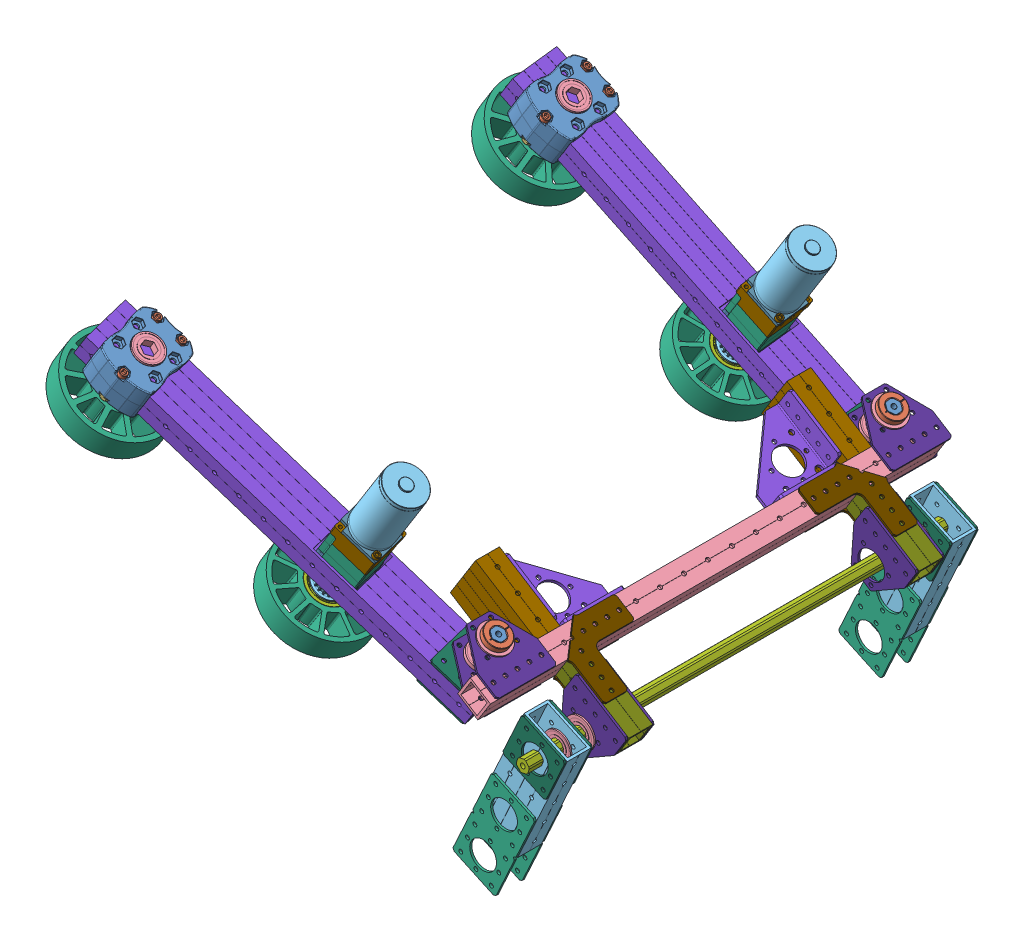
SolidWorks assembly Intake, configuration Default. Lengths in mm. (continued)
Mates (geometry in assembly coordinates): (continued)
- Concentric100: concentric aligned: cylinder of SideBerringGusset-4 through (19.3927 346.1953 456.7755) axis (0.002909 0.001687 -0.999994) radius 14.2875; cylinder of FlangedBerring-13 through (19.3809 346.1885 460.8395) axis (0.002909 0.001687 -0.999994) radius 14.2748
- Coincident266: coincident anti-aligned: plane of SideBerringGusset-4 through (68.234 364.278 454.6621) normal (0.002909 0.001687 -0.999994); plane of FlangedBerring-13 through (34.9523 346.5732 454.5354) normal (-0.002909 -0.001687 0.999994)
- Coincident268: coincident aligned: plane of 1x1x3Stock-3 through (1272.0563 -392.4566 766.975) normal (0.531639 0.846966 0.002975); plane of SideBerringGusset-5 through (67.3386 363.7588 762.46) normal (0.531639 0.846966 0.002975)
- Coincident273: coincident anti-aligned: plane of 1x1x3Stock-3 through (1272.0563 -392.4566 766.975) normal (0.002909 0.001687 -0.999994); plane of SideBerringGusset-5 through (13.5496 397.5144 764.6464) normal (-0.002909 -0.001687 0.999994)
- Coincident279: coincident aligned: plane of 1x1x3Stock-3 through (1272.0563 -392.4566 766.975) normal (0.531639 0.846966 0.002975); plane of SideBerringGusset-6 through (13.4691 397.4677 792.3323) normal (0.531639 0.846966 0.002975)
- Coincident280: coincident aligned: plane of 1x1x3Stock-3 through (67.258 363.7121 790.1458) normal (0.846966 -0.531645 0.001567); plane of SideBerringGusset-6 through (53.7478 342.1953 792.3562) normal (0.846966 -0.531645 0.001567)
- Coincident281: coincident anti-aligned: plane of 1x1x3Stock-3 through (1271.9824 -392.4994 792.3749) normal (-0.002909 -0.001687 0.999994); plane of SideBerringGusset-6 through (67.258 363.7121 790.1458) normal (0.002909 0.001687 -0.999994)
- Coincident282: coincident aligned: plane of SideBerringGusset-5 through (53.8349 342.2459 762.3844) normal (0.846966 -0.531645 0.001567); plane of SideBerringGusset-6 through (53.7478 342.1953 792.3562) normal (0.846966 -0.531645 0.001567)
- Concentric106: concentric anti-aligned: cylinder of SideBerringGusset-6 through (18.4168 345.6295 792.2592) axis (0.002909 0.001687 -0.999994) radius 14.2875; cylinder of FlangedBerring-15 through (18.4353 345.6402 785.9093) axis (-0.002909 -0.001687 0.999994) radius 14.2748
- Coincident317: coincident anti-aligned: plane of SideBerringGusset-6 through (67.2514 363.7083 792.4318) normal (-0.002909 -0.001687 0.999994); plane of FlangedBerring-15 through (18.3906 361.1869 792.2854) normal (0.002909 0.001687 -0.999994)
- Coincident320: coincident: line of SideBerringGusset-4 through (67.0795 362.4455 456.9416) axis (-0.531639 -0.846966 -0.002975); plane of 1x1x3Stock-5 through (68.1534 364.2313 482.3479) normal (0.846966 -0.531645 0.001567)
- Coincident321: coincident aligned: plane of SideBerringGusset-4 through (14.445 398.0335 456.8485) normal (0.531639 0.846966 0.002975); plane of 1x1x3Stock-5 through (1272.9517 -391.9375 459.1771) normal (0.531639 0.846966 0.002975)
- Coincident322: coincident anti-aligned: plane of SideBerringGusset-7 through (68.1534 364.2313 482.3479) normal (0.002909 0.001687 -0.999994); plane of 1x1x3Stock-5 through (1272.8778 -391.9803 484.577) normal (-0.002909 -0.001687 0.999994)
- Coincident323: coincident anti-aligned: plane of SideBerringGusset-4 through (68.2273 364.2741 456.948) normal (-0.002909 -0.001687 0.999994); plane of 1x1x3Stock-5 through (1272.9517 -391.9375 459.1771) normal (0.002909 0.001687 -0.999994)
- Coincident324: coincident aligned: plane of SideBerringGusset-7 through (54.6431 342.7145 484.5583) normal (0.846966 -0.531645 0.001567); plane of 1x1x3Stock-5 through (68.1534 364.2313 482.3479) normal (0.846966 -0.531645 0.001567)
- Coincident332: coincident aligned: plane of 1x1x3Stock-3 through (1271.9824 -392.4994 792.3749) normal (-0.002909 -0.001687 0.999994); plane of PlusGussetHalved-7 through (-22.7562 387.5263 789.9241) normal (-0.002909 -0.001687 0.999994)
- Coincident334: coincident aligned: plane of 1x1x3Stock-5 through (1272.8778 -391.9803 484.577) normal (-0.002909 -0.001687 0.999994); plane of PlusGussetHalved-8 through (-7.1419 411.4945 482.2086) normal (-0.002909 -0.001687 0.999994)
- Coincident337: coincident anti-aligned: plane of 1x1x3Stock-5 through (1259.4481 -413.4504 459.1016) normal (-0.531639 -0.846966 -0.002975); plane of PlusGussetHalved-9 through (-20.4057 390.1206 399.7105) normal (0.531639 0.846966 0.002975)
- Coincident339: coincident: plane of 1x1x3Stock-5 through (1272.8778 -391.9803 484.577) normal (-0.002909 -0.001687 0.999994); line of PlusGussetHalved-9 through (24.6071 358.8772 482.2122) axis (-0.846966 0.531645 -0.001567)
- Parallel21: parallel aligned: line of SideBerringGusset-8 through (-32.3305 394.9636 383.5065) axis (0.846966 -0.531645 0.001567); line of SideBerringGusset-9 through (-16.3962 420.3488 383.5957) axis (0.846966 -0.531645 0.001567)
- Coincident358: coincident aligned: plane of SideBerringGusset-8 through (-31.1151 396.8997 383.5133) normal (0.002909 0.001687 -0.999994); plane of SideBerringGusset-9 through (-16.3962 420.3488 383.5957) normal (0.002909 0.001687 -0.999994)
- Concentric111: concentric anti-aligned: cylinder of SideBerringGusset-9 through (-29.9341 428.7352 415.3206) axis (-0.531639 -0.846966 -0.002975) radius 14.2875; cylinder of FlangedBerring-19 through (-33.31 423.3569 415.3017) axis (0.531639 0.846966 0.002975) radius 14.2748
- Coincident361: coincident anti-aligned: plane of SideBerringGusset-9 through (4.932 406.738 447.1351) normal (0.531639 0.846966 0.002975); plane of FlangedBerring-19 through (-16.9015 420.5628 412.997) normal (-0.531639 -0.846966 -0.002975)
- Concentric113: concentric aligned: cylinder of SideBerringGusset-8 through (-44.6531 405.2861 415.2383) axis (-0.531639 -0.846966 -0.002975) radius 14.2875; cylinder of FlangedBerring-21 through (-42.4925 408.7281 415.2504) axis (-0.531639 -0.846966 -0.002975) radius 14.2748
- Coincident364: coincident anti-aligned: plane of SideBerringGusset-8 through (-11.0022 381.3527 447.046) normal (-0.531639 -0.846966 -0.002975); plane of FlangedBerring-21 through (-59.01 411.5948 416.3956) normal (0.531639 0.846966 0.002975)
- Concentric119: concentric aligned: circle of FlangedBerring-19; cylinder of HexShaft3.5in-1 through (-72.9769 360.1627 415.0798) axis (0.531639 0.846966 0.002975) radius 2.55
- Concentric121: concentric anti-aligned: cylinder of FlangedBerring-19 through (-33.31 423.3569 415.3017) axis (0.531639 0.846966 0.002975) radius 14.2748; cylinder of ShaftCollar-1 through (-25.7142 435.4579 415.3442) axis (-0.531639 -0.846966 -0.002975) radius 12.7
- Coincident369: coincident aligned: plane of HexShaft3.5in-1 through (9.7625 412.8851 501.9282) normal (0.531639 0.846966 0.002975); plane of ShaftCollar-1 through (-25.7142 435.4579 415.3442) normal (0.531639 0.846966 0.002975)
- Coincident370: coincident anti-aligned: plane of FlangedBerring-19 through (-18.4513 423.4084 413.4285) normal (0.531639 0.846966 0.002975); plane of ShaftCollar-1 through (-29.0901 430.0797 415.3254) normal (-0.531639 -0.846966 -0.002975)
- Coincident371: coincident anti-aligned: plane of FlangedBerring-21 through (-52.0763 405.3706 415.7019) normal (-0.531639 -0.846966 -0.002975); plane of 1_4inSpacer-1 through (-46.7124 402.0053 415.2267) normal (0.531639 0.846966 0.002975)
- Coincident374: coincident anti-aligned: plane of ShaftCollar-2 through (-68.829 369.2498 416.5354) normal (0.531639 0.846966 0.002975); plane of Arm-5/FlangedBerring-1 through (-58.7069 362.8812 420.8103) normal (-0.531639 -0.846966 -0.002975)
- Concentric124: concentric aligned: cylinder of ShaftCollar-2 through (-68.829 369.2498 416.5354) axis (-0.531639 -0.846966 -0.002975) radius 12.7; cylinder of Arm-5/FlangedBerring-1 through (-64.6091 375.9726 416.559) axis (-0.531639 -0.846966 -0.002975) radius 15.5575
- Coincident375: coincident anti-aligned: plane of 1_4inSpacer-1 through (-50.0883 396.6271 415.2079) normal (-0.531639 -0.846966 -0.002975); plane of Arm-5/FlangedBerring-2 through (-60.8273 403.3704 414.5071) normal (0.531639 0.846966 0.002975)
- Concentric125: concentric aligned: cylinder of FlangedBerring-21 through (-42.4925 408.7281 415.2504) axis (-0.531639 -0.846966 -0.002975) radius 14.2748; cylinder of 1_4inSpacer-1 through (-46.7124 402.0053 415.2267) axis (-0.531639 -0.846966 -0.002975) radius 9.75
- Concentric126: concentric anti-aligned: cylinder of 1_4inSpacer-1 through (-46.7124 402.0053 415.2267) axis (-0.531639 -0.846966 -0.002975) radius 9.75; cylinder of Arm-5/FlangedBerring-2 through (-54.3082 389.9043 415.1842) axis (0.531639 0.846966 0.002975) radius 15.5575
- Concentric128: concentric aligned: cylinder of FlangedBerring-11 through (-34.5292 422.6501 834.3994) axis (0.531639 0.846966 0.002975) radius 15.5575; cylinder of HexShaft3.5in-2 through (-74.1961 359.4558 834.1774) axis (0.531639 0.846966 0.002975) radius 2.55
- Concentric129: concentric anti-aligned: cylinder of ShaftCollar-3 through (-26.9334 434.7511 834.4419) axis (-0.531639 -0.846966 -0.002975) radius 12.7; cylinder of HexShaft3.5in-2 through (-74.1961 359.4558 834.1774) axis (0.531639 0.846966 0.002975) radius 2.55
- Coincident379: coincident aligned: plane of ShaftCollar-3 through (-26.9334 434.7511 834.4419) normal (0.531639 0.846966 0.002975); plane of HexShaft3.5in-2 through (8.5433 412.1783 921.0259) normal (0.531639 0.846966 0.002975)
- Coincident380: coincident anti-aligned: plane of FlangedBerring-11 through (-19.5814 422.6423 833.4726) normal (0.531639 0.846966 0.002975); plane of ShaftCollar-3 through (-30.3093 429.3729 834.423) normal (-0.531639 -0.846966 -0.002975)
- Concentric134: concentric aligned: cylinder of Arm-3/FlangedBerring-1 through (-65.692 375.1797 835.7901) axis (-0.531639 -0.846966 -0.002975) radius 15.5575; cylinder of ShaftCollar-5 through (-69.9119 368.4569 835.7665) axis (-0.531639 -0.846966 -0.002975) radius 12.7
- Coincident383: coincident anti-aligned: plane of Arm-3/FlangedBerring-1 through (-59.457 361.884 838.7299) normal (-0.531639 -0.846966 -0.002975); plane of ShaftCollar-5 through (-69.9119 368.4569 835.7665) normal (0.531639 0.846966 0.002975)
- Concentric135: concentric aligned: cylinder of FlangedBerring-12 through (-43.7116 408.0213 834.348) axis (-0.531639 -0.846966 -0.002975) radius 15.5575; circle of 1_4inSpacer-3
- Coincident385: coincident anti-aligned: plane of FlangedBerring-12 through (-51.6438 403.5868 846.2522) normal (-0.531639 -0.846966 -0.002975); plane of 1_4inSpacer-3 through (-47.9315 401.2985 834.3244) normal (0.531639 0.846966 0.002975)
- Concentric136: concentric anti-aligned: cylinder of Arm-3/FlangedBerring-2 through (-55.5273 389.1975 834.2819) axis (0.531639 0.846966 0.002975) radius 15.5575; cylinder of FlangedBerring-12 through (-43.7116 408.0213 834.348) axis (-0.531639 -0.846966 -0.002975) radius 14.2748
- Coincident387: coincident anti-aligned: plane of Arm-3/FlangedBerring-2 through (-62.0501 402.6611 834.9731) normal (0.531639 0.846966 0.002975); plane of 1_4inSpacer-3 through (-51.3074 395.9203 834.3055) normal (-0.531639 -0.846966 -0.002975)
- Coincident388: coincident anti-aligned: plane of SideBerringGusset-2 through (2.6823 404.202 802.7263) normal (-0.531639 -0.846966 -0.002975); plane of 1x1x19Stock-2 through (-21.9893 415.8744 1888.5304) normal (0.531639 0.846966 0.002975)
- Coincident389: coincident aligned: plane of SideBerringGusset-2 through (2.4976 404.0949 866.226) normal (0.846966 -0.531645 0.001567); plane of 1x1x19Stock-2 through (-0.4764 402.3707 1888.5702) normal (0.846966 -0.531645 0.001567)
- Coincident390: coincident: line of SideBerringGusset-3 through (-12.0429 380.7493 804.8029) axis (-0.002909 -0.001687 0.999994); plane of 1x1x19Stock-2 through (-0.4764 402.3707 1888.5702) normal (0.846966 -0.531645 0.001567)
- Concentric137: concentric aligned: circle of SideBerringGusset-2; cylinder of 1x1x19Stock-2 through (-8.2404 410.8575 859.8561) axis (-0.531639 -0.846966 -0.002975) radius 2.0701
- Coincident392: coincident aligned: plane of PlusGussetHalved-7 through (-11.9628 380.7958 777.2441) normal (0.846966 -0.531645 0.001567); plane of 1x1x19Stock-2 through (-0.4764 402.3707 1888.5702) normal (0.846966 -0.531645 0.001567)
- Coincident395: coincident anti-aligned: plane of SideBerringGusset-3 through (-11.0061 382.582 866.1504) normal (0.531639 0.846966 0.002975); plane of 1x1x19Stock-2 through (-35.493 394.3615 1888.4548) normal (-0.531639 -0.846966 -0.002975)
- Coincident396: coincident anti-aligned: plane of PlusGussetHalved-7 through (-80.5569 426.5517 777.1217) normal (0.531639 0.846966 0.002975); plane of 1x1x19Stock-2 through (-35.493 394.3615 1888.4548) normal (-0.531639 -0.846966 -0.002975)
- Coincident398: coincident: line of SideBerringGusset-9 through (-17.6115 418.4127 383.5889) axis (0.846966 -0.531645 0.001567); plane of 1x1x19Stock-2 through (-21.9893 415.8744 1888.5304) normal (0.531639 0.846966 0.002975)
- Coincident399: coincident aligned: plane of SideBerringGusset-9 through (5.1168 406.8451 383.6355) normal (0.846966 -0.531645 0.001567); plane of 1x1x19Stock-2 through (-0.4764 402.3707 1888.5702) normal (0.846966 -0.531645 0.001567)
- Coincident400: coincident aligned: plane of SideBerringGusset-8 through (-9.6022 383.396 383.5531) normal (0.846966 -0.531645 0.001567); plane of 1x1x19Stock-2 through (-0.4764 402.3707 1888.5702) normal (0.846966 -0.531645 0.001567)
- Concentric138: concentric aligned: cylinder of SideBerringGusset-9 through (-5.6951 413.5648 402.6655) axis (-0.531639 -0.846966 -0.002975) radius 2.0701; cylinder of 1x1x19Stock-2 through (-6.9104 411.6287 402.6587) axis (-0.531639 -0.846966 -0.002975) radius 2.0701
- Coincident402: coincident anti-aligned: plane of PlusGussetHalved-8 through (-6.9021 411.6335 399.7861) normal (-0.531639 -0.846966 -0.002975); plane of 1x1x19Stock-2 through (-21.9893 415.8744 1888.5304) normal (0.531639 0.846966 0.002975)
- Coincident403: coincident anti-aligned: plane of PlusGussetHalved-9 through (-20.4057 390.1206 399.7105) normal (0.531639 0.846966 0.002975); plane of 1x1x19Stock-2 through (-35.493 394.3615 1888.4548) normal (-0.531639 -0.846966 -0.002975)
- Coincident404: coincident aligned: plane of PlusGussetHalved-9 through (-11.0674 381.3149 469.4462) normal (0.846966 -0.531645 0.001567); plane of 1x1x19Stock-2 through (-0.4764 402.3707 1888.5702) normal (0.846966 -0.531645 0.001567)
- Coincident405: coincident anti-aligned: plane of 1x1x3Stock-5 through (-3.1003 394.0076 469.4908) normal (-0.846966 0.531645 -0.001567); plane of 1x1x19Stock-2 through (-0.4764 402.3707 1888.5702) normal (0.846966 -0.531645 0.001567)
- Coincident406: coincident anti-aligned: plane of 1x1x3Stock-3 through (-3.9956 393.4884 777.2887) normal (-0.846966 0.531645 -0.001567); plane of 1x1x19Stock-2 through (-0.4764 402.3707 1888.5702) normal (0.846966 -0.531645 0.001567)
- Coincident408: coincident anti-aligned: plane of SideBerringGusset-8 through (-9.7869 383.2889 447.0528) normal (0.531639 0.846966 0.002975); plane of 1x1x19Stock-2 through (-35.493 394.3615 1888.4548) normal (-0.531639 -0.846966 -0.002975)
- Coincident409: coincident aligned: plane of FaceBerringMountGussetHalved-1 through (28.9197 303.0177 432.2979) normal (0.907821 -0.419354 0.001934); plane of FaceBerringMountGussetHalved-2 through (29 303.0643 404.6883) normal (0.907821 -0.419354 0.001934)
- Coincident410: coincident: line of 1x2x5HoledStock-2 through (-21.9348 253.3803 406.9963) axis (0.419348 0.907821 0.002751); plane of FaceBerringMountGussetHalved-2 through (-12.8173 333.3852 407.1578) normal (-0.002909 -0.001687 0.999994)
- Coincident411: coincident anti-aligned: plane of 1x2x5HoledStock-2 through (54.3074 357.9793 432.7184) normal (-0.002909 -0.001687 0.999994); plane of FaceBerringMountGussetHalved-1 through (-12.891 333.3425 432.4814) normal (0.002909 0.001687 -0.999994)
- Coincident412: coincident aligned: plane of FaceBerringMountGussetHalved-1 through (8.2988 379.2254 434.9065) normal (0.419348 0.907821 0.002751); plane of FaceBerringMountGussetHalved-2 through (8.3791 379.2719 407.2968) normal (0.419348 0.907821 0.002751)
- Coincident413: coincident: line of 1x2x5HoledStock-2 through (52.0681 359.083 409.8537) axis (-0.002909 -0.001687 0.999994); plane of FaceBerringMountGussetHalved-2 through (8.3791 379.2719 407.2968) normal (0.419348 0.907821 0.002751)
- Coincident414: coincident aligned: plane of 1x2x5HoledStock-2 through (54.3074 357.9793 432.7184) normal (0.907821 -0.419354 0.001934); plane of FaceBerringMountGussetHalved-2 through (29 303.0643 404.6883) normal (0.907821 -0.419354 0.001934)
- Coincident415: coincident anti-aligned: plane of ? through (-51.9684 -15.5546 848.5224) normal (0 0 -1); plane of ? through (-1.2954 34.9914 848.5224) normal (0 0 1)
- Coincident421: coincident anti-aligned: plane of 1x2x5HoledStock-2 through (54.3074 357.9793 432.7184) normal (-0.002909 -0.001687 0.999994); plane of FaceBerringMountGusset-10 through (-23.6401 309.7694 432.4104) normal (0.002909 0.001687 -0.999994)
- Coincident422: coincident aligned: plane of 1x2x5HoledStock-2 through (54.3074 357.9793 432.7184) normal (0.907821 -0.419354 0.001934); plane of FaceBerringMountGusset-10 through (22.2399 288.5689 434.7941) normal (0.907821 -0.419354 0.001934)
- Coincident423: coincident anti-aligned: plane of 1x2x5HoledStock-2 through (54.3813 358.0222 407.3186) normal (0.002909 0.001687 -0.999994); plane of FaceBerringMountGusset-11 through (-23.5662 309.8122 407.0105) normal (-0.002909 -0.001687 0.999994)
- Coincident424: coincident aligned: plane of 1x2x5HoledStock-2 through (54.3074 357.9793 432.7184) normal (0.907821 -0.419354 0.001934); plane of FaceBerringMountGusset-11 through (22.3205 288.6156 407.1083) normal (0.907821 -0.419354 0.001934)
- Coincident427: coincident aligned: plane of FaceBerringMountGusset-10 through (-20.2593 196.5648 434.5153) normal (-0.419348 -0.907821 -0.002751); plane of FaceBerringMountGusset-11 through (-20.1788 196.6115 406.8295) normal (-0.419348 -0.907821 -0.002751)
- Distance1: distance = 50.8 mm aligned: plane of FaceBerringMountGusset-10 through (-20.2593 196.5648 434.5153) normal (-0.419348 -0.907821 -0.002751); plane of 1x2x5HoledStock-2 through (1.0502 242.686 432.3691) normal (-0.419348 -0.907821 -0.002751)
- Concentric141: concentric anti-aligned: cylinder of FaceBerringMountGussetHalved-1 through (19.4564 346.2322 434.8833) axis (0.002909 0.001687 -0.999994) radius 14.2875; cylinder of FlangedBerring-22 through (19.4749 346.2429 428.5333) axis (-0.002909 -0.001687 0.999994) radius 14.2748
- Coincident429: coincident anti-aligned: plane of FaceBerringMountGussetHalved-1 through (-12.8976 333.3386 434.7674) normal (-0.002909 -0.001687 0.999994); plane of FlangedBerring-22 through (19.4302 361.7897 434.9094) normal (0.002909 0.001687 -0.999994)
- Coincident430: coincident: line of PlusGussetHalved-8 through (4.7073 406.6076 524.399) axis (0.002909 0.001687 -0.999994); plane of 1x1x19Stock-2 through (-0.4764 402.3707 1888.5702) normal (0.846966 -0.531645 0.001567)
- Coincident431: coincident aligned: plane of SideBerringGusset-7 through (14.3644 397.9869 484.5344) normal (0.531639 0.846966 0.002975); plane of 1x1x3Stock-5 through (1272.9517 -391.9375 459.1771) normal (0.531639 0.846966 0.002975)
- Concentric143: concentric anti-aligned: cylinder of FlangedBerring-23 through (18.3429 345.5866 817.6591) axis (0.002909 0.001687 -0.999994) radius 14.2748; cylinder of FaceBerringMountGussetHalved-6 through (18.3614 345.5974 811.3091) axis (-0.002909 -0.001687 0.999994) radius 14.2875
- Distance2: distance = 50.8 mm aligned: plane of FaceBerringMountGusset-12 through (-69.8467 218.3302 810.8379) normal (-0.419348 -0.907821 -0.002751); plane of 1x2x5HoledStock-4 through (-48.5504 264.4437 813.2636) normal (-0.419348 -0.907821 -0.002751)
- Coincident432: coincident anti-aligned: plane of FaceBerringMountGussetHalved-6 through (29.5124 312.6004 813.5719) normal (-0.002909 -0.001687 0.999994); plane of 1x2x5HoledStock-4 through (4.7068 379.737 813.613) normal (0.002909 0.001687 -0.999994)
- Coincident433: coincident aligned: plane of FaceBerringMountGussetHalved-5 through (-20.7628 324.728 841.3101) normal (-0.907821 0.419354 -0.001934); plane of FaceBerringMountGussetHalved-6 through (-20.6825 324.7746 813.7005) normal (-0.907821 0.419354 -0.001934)
- Coincident434: coincident aligned: plane of FaceBerringMountGusset-12 through (-69.8467 218.3302 810.8379) normal (-0.419348 -0.907821 -0.002751); plane of FaceBerringMountGusset-13 through (-69.9272 218.2835 838.5237) normal (-0.419348 -0.907821 -0.002751)
- Coincident435: coincident: plane of FaceBerringMountGussetHalved-5 through (29.4387 312.5577 838.8956) normal (0.002909 0.001687 -0.999994); line of 1x2x5HoledStock-4 through (-25.5655 253.7494 838.6364) axis (0.419348 0.907821 0.002751)
- Coincident436: coincident anti-aligned: plane of FaceBerringMountGusset-13 through (18.4588 289.0909 838.9003) normal (0.002909 0.001687 -0.999994); plane of 1x2x5HoledStock-4 through (4.6329 379.6942 839.0129) normal (-0.002909 -0.001687 0.999994)
- Coincident437: coincident aligned: plane of FaceBerringMountGusset-12 through (-27.3474 310.3343 811.1167) normal (-0.907821 0.419354 -0.001934); plane of 1x2x5HoledStock-4 through (4.7068 379.737 813.613) normal (-0.907821 0.419354 -0.001934)
- Coincident438: coincident aligned: plane of FaceBerringMountGussetHalved-5 through (-20.7628 324.728 841.3101) normal (-0.907821 0.419354 -0.001934); plane of 1x2x5HoledStock-4 through (4.7068 379.737 813.613) normal (-0.907821 0.419354 -0.001934)
- Coincident439: coincident aligned: plane of FaceBerringMountGussetHalved-5 through (50.6351 358.4444 839.0346) normal (0.419348 0.907821 0.002751); plane of FaceBerringMountGussetHalved-6 through (50.7154 358.491 811.425) normal (0.419348 0.907821 0.002751)
- Coincident440: coincident: plane of FaceBerringMountGussetHalved-5 through (50.6351 358.4444 839.0346) normal (0.419348 0.907821 0.002751); line of 1x2x5HoledStock-4 through (6.9461 378.6333 836.4778) axis (0.002909 0.001687 -0.999994)
- Coincident441: coincident anti-aligned: plane of FaceBerringMountGusset-12 through (18.5326 289.1338 813.5004) normal (-0.002909 -0.001687 0.999994); plane of 1x2x5HoledStock-4 through (4.7068 379.737 813.613) normal (0.002909 0.001687 -0.999994)
- Coincident442: coincident aligned: plane of FaceBerringMountGusset-13 through (-27.428 310.2876 838.8025) normal (-0.907821 0.419354 -0.001934); plane of 1x2x5HoledStock-4 through (4.7068 379.737 813.613) normal (-0.907821 0.419354 -0.001934)
- Coincident443: coincident anti-aligned: plane of FlangedBerring-23 through (14.384 360.6378 811.3229) normal (-0.002909 -0.001687 0.999994); plane of FaceBerringMountGussetHalved-6 through (29.5191 312.6042 811.286) normal (0.002909 0.001687 -0.999994)
- Distance3: distance = 381 mm anti-aligned: plane of FaceBerringMountGusset-12 through (18.5326 289.1338 813.5004) normal (-0.002909 -0.001687 0.999994); plane of FaceBerringMountGusset-10 through (-23.6401 309.7694 432.4104) normal (0.002909 0.001687 -0.999994)
- Parallel24: parallel aligned: plane of FaceBerringMountGussetHalved-1 through (28.9197 303.0177 432.2979) normal (0.907821 -0.419354 0.001934); plane of FaceBerringMountGussetHalved-6 through (50.7154 358.491 811.425) normal (0.907821 -0.419354 0.001934)
- Concentric149: concentric anti-aligned: cylinder of FlangedBerring-22 through (19.4749 346.2429 428.5333) axis (-0.002909 -0.001687 0.999994) radius 15.5575; cylinder of FlangedBerring-23 through (18.3429 345.5866 817.6591) axis (0.002909 0.001687 -0.999994) radius 15.5575
- Concentric150: concentric anti-aligned: cylinder of FlangedBerring-15 through (18.4353 345.6402 785.9093) axis (-0.002909 -0.001687 0.999994) radius 15.5575; cylinder of FlangedBerring-23 through (18.3429 345.5866 817.6591) axis (0.002909 0.001687 -0.999994) radius 15.5575
- Concentric152: concentric anti-aligned: cylinder of FaceBerringMountGussetHalved-2 through (19.5367 346.2788 407.2736) axis (0.002909 0.001687 -0.999994) radius 14.2875; cylinder of HexShaft-3 through (19.5675 346.2966 396.7073) axis (-0.002909 -0.001687 0.999994) radius 2.55
- Distance4: distance = 12.7 mm aligned: plane of HexShaft-3 through (18.2375 345.5255 853.9047) normal (-0.002909 -0.001687 0.999994); plane of FaceBerringMountGussetHalved-5 through (29.4321 312.5538 841.1816) normal (-0.002909 -0.001687 0.999994)
- Distance5: distance = 19.05 mm anti-aligned: plane of FaceBerringMountGussetHalved-6 through (29.5191 312.6042 811.286) normal (0.002909 0.001687 -0.999994); plane of SideBerringGusset-6 through (67.2514 363.7083 792.4318) normal (-0.002909 -0.001687 0.999994)
- Coincident458: coincident aligned: plane of PlusGussetHalved-7 through (-11.9628 380.7958 777.2441) normal (0.846966 -0.531645 0.001567); plane of PlusGussetHalved-12 through (2.7562 404.2449 777.3265) normal (0.846966 -0.531645 0.001567)
- Coincident459: coincident aligned: plane of 1x1x3Stock-3 through (1272.0563 -392.4566 766.975) normal (0.002909 0.001687 -0.999994); plane of PlusGussetHalved-12 through (-7.9633 411.0182 764.6066) normal (0.002909 0.001687 -0.999994)
- Coincident460: coincident anti-aligned: plane of 1x1x3Stock-3 through (1272.0563 -392.4566 766.975) normal (0.531639 0.846966 0.002975); plane of PlusGussetHalved-12 through (-67.0533 448.0646 777.1973) normal (-0.531639 -0.846966 -0.002975)
- Coincident461: coincident anti-aligned: plane of 1x1x19Stock-2 through (-21.9893 415.8744 1888.5304) normal (0.531639 0.846966 0.002975); plane of PlusGussetHalved-12 through (-67.0533 448.0646 777.1973) normal (-0.531639 -0.846966 -0.002975)
- Distance6: distance = 82.55 mm aligned: plane of 1x1x19Stock-2 through (-32.5375 396.0751 872.4606) normal (-0.002909 -0.001687 0.999994); plane of 1x1x3Stock-3 through (1271.9824 -392.4994 792.3749) normal (-0.002909 -0.001687 0.999994)
- Coincident464: coincident anti-aligned: plane of 1x1x19Stock-2 through (-21.9893 415.8744 1888.5304) normal (-0.846966 0.531645 -0.001567); plane of CornerGusset-1 through (-32.2604 396.2357 777.2111) normal (0.846966 -0.531645 0.001567)
- Coincident465: coincident aligned: plane of 1x1x19Stock-2 through (-21.9893 415.8744 1888.5304) normal (0.531639 0.846966 0.002975); plane of CornerGusset-1 through (-18.7379 417.7596 770.8097) normal (0.531639 0.846966 0.002975)
- Coincident467: coincident anti-aligned: plane of 1x1x19Stock-2 through (-21.9893 415.8744 1888.5304) normal (-0.846966 0.531645 -0.001567); plane of CornerGusset-2 through (-31.3737 396.7498 472.4128) normal (0.846966 -0.531645 0.001567)
- Coincident468: coincident aligned: plane of 1x1x19Stock-2 through (-21.9893 415.8744 1888.5304) normal (0.531639 0.846966 0.002975); plane of CornerGusset-2 through (-18.0729 418.1451 542.211) normal (0.531639 0.846966 0.002975)
- Coincident469: coincident aligned: plane of CornerGusset-1 through (-77.8098 454.8165 777.1774) normal (0.531639 0.846966 0.002975); plane of 1x2x3Stock-1 through (-18.8306 417.7058 802.6865) normal (0.531639 0.846966 0.002975)
- Coincident470: coincident anti-aligned: plane of CornerGusset-1 through (-32.2604 396.2357 777.2111) normal (-0.002909 -0.001687 0.999994); plane of 1x2x3Stock-1 through (-45.764 374.7228 777.1355) normal (0.002909 0.001687 -0.999994)
- Coincident471: coincident anti-aligned: plane of 1x1x19Stock-2 through (-21.9893 415.8744 1888.5304) normal (-0.846966 0.531645 -0.001567); plane of 1x2x3Stock-1 through (-32.2973 396.2143 789.911) normal (0.846966 -0.531645 0.001567)
- Coincident478: coincident aligned: plane of 1x1x19Stock-2 through (-21.9893 415.8744 1888.5304) normal (0.531639 0.846966 0.002975); plane of 1x2x3Stock-2 through (-17.8701 418.2627 472.4884) normal (0.531639 0.846966 0.002975)
- Coincident479: coincident anti-aligned: plane of CornerGusset-2 through (-31.3737 396.7498 472.4128) normal (0.002909 0.001687 -0.999994); plane of 1x2x3Stock-2 through (-44.8774 375.2369 472.3373) normal (-0.002909 -0.001687 0.999994)
- Coincident480: coincident: line of 1x1x19Stock-2 through (-24.4223 407.581 389.9008) axis (-0.002909 -0.001687 0.999994); plane of 1x2x3Stock-2 through (-31.3368 396.7712 459.7129) normal (0.846966 -0.531645 0.001567)
- Coincident481: coincident: line of SideBerringGusset-9 through (-16.5809 420.2417 447.0953) axis (-0.531639 -0.846966 -0.002975); plane of 1x2x3Stock-2 through (-44.8035 375.2797 446.9374) normal (0.002909 0.001687 -0.999994)
- Coincident482: coincident: line of SideBerringGusset-2 through (-18.8306 417.7058 802.6865) axis (0.531639 0.846966 0.002975); plane of 1x2x3Stock-1 through (-45.8379 374.68 802.5354) normal (-0.002909 -0.001687 0.999994)
- LimitAngle4: limit planar angle = 0.195067 rad aligned: line of 1x2x3Stock-1 through (-110.3767 415.1913 802.416) axis (0.846966 -0.531645 0.001567); line of Arm-3/1x2x16StockSlotted-1 through (-374.1271 593.8055 884.0647) axis (0.831467 -0.521235 -0.192294)
- LimitAngle5: limit planar angle = 0.087266 rad aligned: line of Arm-5/1x2x16StockSlotted-1 through (-385.4179 572.3421 474.4795) axis (0.843997 -0.529475 -0.085594); line of 1x2x3Stock-2 through (-109.3423 415.7911 446.818) axis (0.846966 -0.531645 0.001567)
